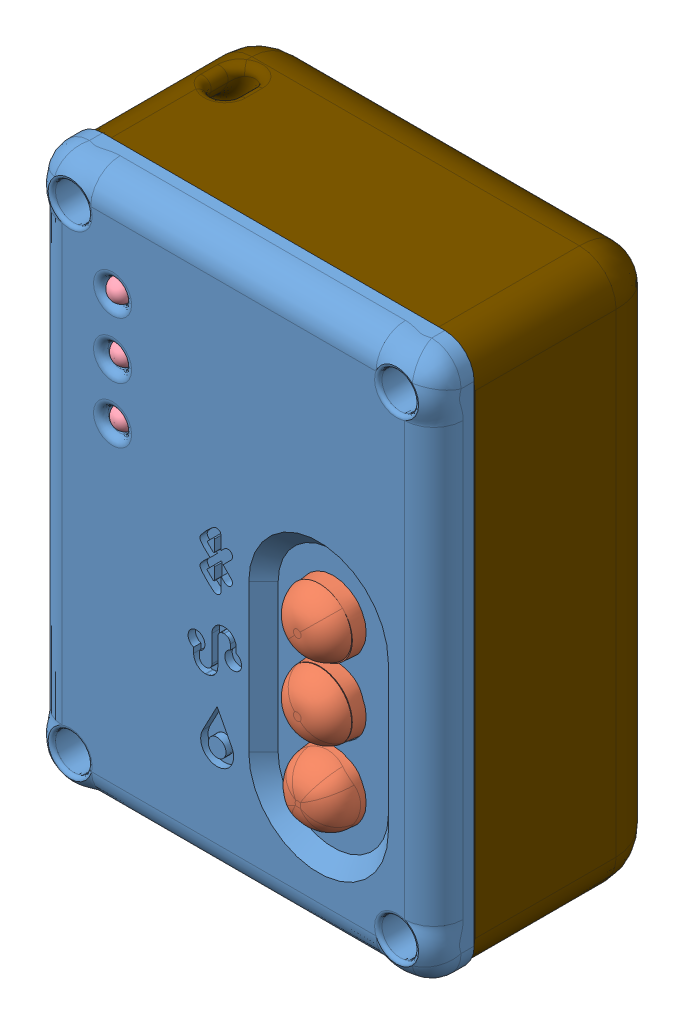
SolidWorks assembly tracker, configuration По умолчанию. Lengths in mm.
Overall size (452.18 452.18 291.35).
146 component instances, 27 part files, 100 mates.
Components (placement in the parent):
- YAAJ_BluePill.step-1: YAAJ_BluePill.step [По умолчанию] at origin size (22.6 53 12.5)
- Stiftleiste, RM 2,54 mm - 6-3 mm, gerade - 1 x 20 - schwarz.stp-3: Stiftleiste, RM 2,54 mm - 6-3 mm, gerade - 1 x 20 - schwarz.stp [По умолчанию] at (13.97 1.27 1.6) x (0 -1 0) z (0 0 1) size (50.8 2.54 11.57)
  - Stiftleiste, RM 2,54 mm - Tr_ger - 1 x 20 - schwarz.stp-1: Stiftleiste, RM 2,54 mm - Tr_ger - 1 x 20 - schwarz.stp [По умолчанию] at origin size (50.8 2.54 2.54)
  - Stiftleiste, RM 2,54 mm - Stift -  6-3 mm, gerade.stp-1: Stiftleiste, RM 2,54 mm - Stift -  6-3 mm, gerade.stp [По умолчанию] at (1.27 1.27 -3) size (1.03 1.03 11.57)
  - Stiftleiste, RM 2,54 mm - Stift -  6-3 mm, gerade.stp-2: Stiftleiste, RM 2,54 mm - Stift -  6-3 mm, gerade.stp [По умолчанию] at (46.99 1.27 -3) size (1.03 1.03 11.57)
  - Stiftleiste, RM 2,54 mm - Stift -  6-3 mm, gerade.stp-3: Stiftleiste, RM 2,54 mm - Stift -  6-3 mm, gerade.stp [По умолчанию] at (44.45 1.27 -3) size (1.03 1.03 11.57)
  - Stiftleiste, RM 2,54 mm - Stift -  6-3 mm, gerade.stp-4: Stiftleiste, RM 2,54 mm - Stift -  6-3 mm, gerade.stp [По умолчанию] at (41.91 1.27 -3) size (1.03 1.03 11.57)
  - Stiftleiste, RM 2,54 mm - Stift -  6-3 mm, gerade.stp-5: Stiftleiste, RM 2,54 mm - Stift -  6-3 mm, gerade.stp [По умолчанию] at (39.37 1.27 -3) size (1.03 1.03 11.57)
  - Stiftleiste, RM 2,54 mm - Stift -  6-3 mm, gerade.stp-6: Stiftleiste, RM 2,54 mm - Stift -  6-3 mm, gerade.stp [По умолчанию] at (36.83 1.27 -3) size (1.03 1.03 11.57)
  - Stiftleiste, RM 2,54 mm - Stift -  6-3 mm, gerade.stp-7: Stiftleiste, RM 2,54 mm - Stift -  6-3 mm, gerade.stp [По умолчанию] at (34.29 1.27 -3) size (1.03 1.03 11.57)
  - Stiftleiste, RM 2,54 mm - Stift -  6-3 mm, gerade.stp-8: Stiftleiste, RM 2,54 mm - Stift -  6-3 mm, gerade.stp [По умолчанию] at (31.75 1.27 -3) size (1.03 1.03 11.57)
  - Stiftleiste, RM 2,54 mm - Stift -  6-3 mm, gerade.stp-9: Stiftleiste, RM 2,54 mm - Stift -  6-3 mm, gerade.stp [По умолчанию] at (29.21 1.27 -3) size (1.03 1.03 11.57)
  - Stiftleiste, RM 2,54 mm - Stift -  6-3 mm, gerade.stp-10: Stiftleiste, RM 2,54 mm - Stift -  6-3 mm, gerade.stp [По умолчанию] at (49.53 1.27 -3) size (1.03 1.03 11.57)
  - Stiftleiste, RM 2,54 mm - Stift -  6-3 mm, gerade.stp-11: Stiftleiste, RM 2,54 mm - Stift -  6-3 mm, gerade.stp [По умолчанию] at (21.59 1.27 -3) size (1.03 1.03 11.57)
  - Stiftleiste, RM 2,54 mm - Stift -  6-3 mm, gerade.stp-12: Stiftleiste, RM 2,54 mm - Stift -  6-3 mm, gerade.stp [По умолчанию] at (19.05 1.27 -3) size (1.03 1.03 11.57)
  - Stiftleiste, RM 2,54 mm - Stift -  6-3 mm, gerade.stp-13: Stiftleiste, RM 2,54 mm - Stift -  6-3 mm, gerade.stp [По умолчанию] at (16.51 1.27 -3) size (1.03 1.03 11.57)
  - Stiftleiste, RM 2,54 mm - Stift -  6-3 mm, gerade.stp-14: Stiftleiste, RM 2,54 mm - Stift -  6-3 mm, gerade.stp [По умолчанию] at (6.35 1.27 -3) size (1.03 1.03 11.57)
  - Stiftleiste, RM 2,54 mm - Stift -  6-3 mm, gerade.stp-15: Stiftleiste, RM 2,54 mm - Stift -  6-3 mm, gerade.stp [По умолчанию] at (13.97 1.27 -3) size (1.03 1.03 11.57)
  - Stiftleiste, RM 2,54 mm - Stift -  6-3 mm, gerade.stp-16: Stiftleiste, RM 2,54 mm - Stift -  6-3 mm, gerade.stp [По умолчанию] at (11.43 1.27 -3) size (1.03 1.03 11.57)
  - Stiftleiste, RM 2,54 mm - Stift -  6-3 mm, gerade.stp-17: Stiftleiste, RM 2,54 mm - Stift -  6-3 mm, gerade.stp [По умолчанию] at (8.89 1.27 -3) size (1.03 1.03 11.57)
  - Stiftleiste, RM 2,54 mm - Stift -  6-3 mm, gerade.stp-18: Stiftleiste, RM 2,54 mm - Stift -  6-3 mm, gerade.stp [По умолчанию] at (26.67 1.27 -3) size (1.03 1.03 11.57)
  - Stiftleiste, RM 2,54 mm - Stift -  6-3 mm, gerade.stp-19: Stiftleiste, RM 2,54 mm - Stift -  6-3 mm, gerade.stp [По умолчанию] at (24.13 1.27 -3) size (1.03 1.03 11.57)
  - Stiftleiste, RM 2,54 mm - Stift -  6-3 mm, gerade.stp-20: Stiftleiste, RM 2,54 mm - Stift -  6-3 mm, gerade.stp [По умолчанию] at (3.81 1.27 -3) size (1.03 1.03 11.57)
- Stiftleiste, RM 2,54 mm - 6-3 mm, gerade - 1 x 20 - schwarz.stp-4: Stiftleiste, RM 2,54 mm - 6-3 mm, gerade - 1 x 20 - schwarz.stp [По умолчанию] at (1.27 -49.53 1.6) x (0 1 0) z (0 0 1) size (50.8 2.54 11.57)
  - Stiftleiste, RM 2,54 mm - Tr_ger - 1 x 20 - schwarz.stp-1: Stiftleiste, RM 2,54 mm - Tr_ger - 1 x 20 - schwarz.stp [По умолчанию] at origin size (50.8 2.54 2.54)
  - Stiftleiste, RM 2,54 mm - Stift -  6-3 mm, gerade.stp-1: Stiftleiste, RM 2,54 mm - Stift -  6-3 mm, gerade.stp [По умолчанию] at (1.27 1.27 -3) size (1.03 1.03 11.57)
  - Stiftleiste, RM 2,54 mm - Stift -  6-3 mm, gerade.stp-2: Stiftleiste, RM 2,54 mm - Stift -  6-3 mm, gerade.stp [По умолчанию] at (46.99 1.27 -3) size (1.03 1.03 11.57)
  - Stiftleiste, RM 2,54 mm - Stift -  6-3 mm, gerade.stp-3: Stiftleiste, RM 2,54 mm - Stift -  6-3 mm, gerade.stp [По умолчанию] at (44.45 1.27 -3) size (1.03 1.03 11.57)
  - Stiftleiste, RM 2,54 mm - Stift -  6-3 mm, gerade.stp-4: Stiftleiste, RM 2,54 mm - Stift -  6-3 mm, gerade.stp [По умолчанию] at (41.91 1.27 -3) size (1.03 1.03 11.57)
  - Stiftleiste, RM 2,54 mm - Stift -  6-3 mm, gerade.stp-5: Stiftleiste, RM 2,54 mm - Stift -  6-3 mm, gerade.stp [По умолчанию] at (39.37 1.27 -3) size (1.03 1.03 11.57)
  - Stiftleiste, RM 2,54 mm - Stift -  6-3 mm, gerade.stp-6: Stiftleiste, RM 2,54 mm - Stift -  6-3 mm, gerade.stp [По умолчанию] at (36.83 1.27 -3) size (1.03 1.03 11.57)
  - Stiftleiste, RM 2,54 mm - Stift -  6-3 mm, gerade.stp-7: Stiftleiste, RM 2,54 mm - Stift -  6-3 mm, gerade.stp [По умолчанию] at (34.29 1.27 -3) size (1.03 1.03 11.57)
  - Stiftleiste, RM 2,54 mm - Stift -  6-3 mm, gerade.stp-8: Stiftleiste, RM 2,54 mm - Stift -  6-3 mm, gerade.stp [По умолчанию] at (31.75 1.27 -3) size (1.03 1.03 11.57)
  - Stiftleiste, RM 2,54 mm - Stift -  6-3 mm, gerade.stp-9: Stiftleiste, RM 2,54 mm - Stift -  6-3 mm, gerade.stp [По умолчанию] at (29.21 1.27 -3) size (1.03 1.03 11.57)
  - Stiftleiste, RM 2,54 mm - Stift -  6-3 mm, gerade.stp-10: Stiftleiste, RM 2,54 mm - Stift -  6-3 mm, gerade.stp [По умолчанию] at (49.53 1.27 -3) size (1.03 1.03 11.57)
  - Stiftleiste, RM 2,54 mm - Stift -  6-3 mm, gerade.stp-11: Stiftleiste, RM 2,54 mm - Stift -  6-3 mm, gerade.stp [По умолчанию] at (21.59 1.27 -3) size (1.03 1.03 11.57)
  - Stiftleiste, RM 2,54 mm - Stift -  6-3 mm, gerade.stp-12: Stiftleiste, RM 2,54 mm - Stift -  6-3 mm, gerade.stp [По умолчанию] at (19.05 1.27 -3) size (1.03 1.03 11.57)
  - Stiftleiste, RM 2,54 mm - Stift -  6-3 mm, gerade.stp-13: Stiftleiste, RM 2,54 mm - Stift -  6-3 mm, gerade.stp [По умолчанию] at (16.51 1.27 -3) size (1.03 1.03 11.57)
  - Stiftleiste, RM 2,54 mm - Stift -  6-3 mm, gerade.stp-14: Stiftleiste, RM 2,54 mm - Stift -  6-3 mm, gerade.stp [По умолчанию] at (6.35 1.27 -3) size (1.03 1.03 11.57)
  - Stiftleiste, RM 2,54 mm - Stift -  6-3 mm, gerade.stp-15: Stiftleiste, RM 2,54 mm - Stift -  6-3 mm, gerade.stp [По умолчанию] at (13.97 1.27 -3) size (1.03 1.03 11.57)
  - Stiftleiste, RM 2,54 mm - Stift -  6-3 mm, gerade.stp-16: Stiftleiste, RM 2,54 mm - Stift -  6-3 mm, gerade.stp [По умолчанию] at (11.43 1.27 -3) size (1.03 1.03 11.57)
  - Stiftleiste, RM 2,54 mm - Stift -  6-3 mm, gerade.stp-17: Stiftleiste, RM 2,54 mm - Stift -  6-3 mm, gerade.stp [По умолчанию] at (8.89 1.27 -3) size (1.03 1.03 11.57)
  - Stiftleiste, RM 2,54 mm - Stift -  6-3 mm, gerade.stp-18: Stiftleiste, RM 2,54 mm - Stift -  6-3 mm, gerade.stp [По умолчанию] at (26.67 1.27 -3) size (1.03 1.03 11.57)
  - Stiftleiste, RM 2,54 mm - Stift -  6-3 mm, gerade.stp-19: Stiftleiste, RM 2,54 mm - Stift -  6-3 mm, gerade.stp [По умолчанию] at (24.13 1.27 -3) size (1.03 1.03 11.57)
  - Stiftleiste, RM 2,54 mm - Stift -  6-3 mm, gerade.stp-20: Stiftleiste, RM 2,54 mm - Stift -  6-3 mm, gerade.stp [По умолчанию] at (3.81 1.27 -3) size (1.03 1.03 11.57)
- pcb_proto_board(40x60) .step-1: pcb_proto_board(40x60) .step [По умолчанию] at (-10.994 5.734 9.14) x (0 -1 0) z (0 0 1) size (60 40 2.1)
- HC-05-1: HC-05 [Default] at (1.6677 -8.4393 11.13) x (0 -1 0) z (-1 0 0) size (42.58 5.8 16)
- Troyka SD card.stp-1: Troyka SD card.stp [По умолчанию] at (-11.7222 -53.8342 13.43) size (26.65 26.3 12.48)
  - SOT23-5.stp-1: SOT23-5.stp [По умолчанию] at (18.8632 22.6732 0.75) x (-1 0 0) z (0 0 1) size (3.1 3.38 1.3)
    - SOT23-5 Geometry.stp-1: SOT23-5 Geometry.stp [По умолчанию] at origin size (3.1 1.8 1.3)
    - leg.stp-1: leg.stp [По умолчанию] at origin size (0.5 0.79 1)
    - leg.stp-2: leg.stp [По умолчанию] at (-0.95 0 0) size (0.5 0.79 1)
    - leg.stp-3: leg.stp [По умолчанию] at (-1.9 0 0) size (0.5 0.79 1)
    - leg.stp-4: leg.stp [По умолчанию] at (0 0.01 0) x (-1 0 0) z (0 0 1) size (0.5 0.79 1)
    - leg.stp-5: leg.stp [По умолчанию] at (1.9 0.01 0) x (-1 0 0) z (0 0 1) size (0.5 0.79 1)
  - SOT23-5-1.stp-1: SOT23-5-1.stp [По умолчанию] at (11.4972 22.8002 0.75) x (-1 0 0) z (0 0 1) size (3.1 3.38 1.3)
    - SOT23-5 Geometry.stp-1: SOT23-5 Geometry.stp [По умолчанию] at origin size (3.1 1.8 1.3)
    - leg.stp-1: leg.stp [По умолчанию] at origin size (0.5 0.79 1)
    - leg.stp-2: leg.stp [По умолчанию] at (-0.95 0 0) size (0.5 0.79 1)
    - leg.stp-3: leg.stp [По умолчанию] at (-1.9 0 0) size (0.5 0.79 1)
    - leg.stp-4: leg.stp [По умолчанию] at (0 0.01 0) x (-1 0 0) z (0 0 1) size (0.5 0.79 1)
    - leg.stp-5: leg.stp [По умолчанию] at (1.9 0.01 0) x (-1 0 0) z (0 0 1) size (0.5 0.79 1)
  - SOT23-5-2.stp-1: SOT23-5-2.stp [По умолчанию] at (15.1802 22.4192 0.75) x (-1 0 0) z (0 0 1) size (3.1 3.38 1.3)
    - SOT23-5 Geometry.stp-1: SOT23-5 Geometry.stp [По умолчанию] at origin size (3.1 1.8 1.3)
    - leg.stp-1: leg.stp [По умолчанию] at origin size (0.5 0.79 1)
    - leg.stp-2: leg.stp [По умолчанию] at (-0.95 0 0) size (0.5 0.79 1)
    - leg.stp-3: leg.stp [По умолчанию] at (-1.9 0 0) size (0.5 0.79 1)
    - leg.stp-4: leg.stp [По умолчанию] at (0 0.01 0) x (-1 0 0) z (0 0 1) size (0.5 0.79 1)
    - leg.stp-5: leg.stp [По умолчанию] at (1.9 0.01 0) x (-1 0 0) z (0 0 1) size (0.5 0.79 1)
  - SOT23-5-3.stp-1: SOT23-5-3.stp [По умолчанию] at (22.6732 7.4332 0.75) x (0 -1 0) z (0 0 1) size (3.1 3.38 1.3)
    - SOT23-5 Geometry.stp-1: SOT23-5 Geometry.stp [По умолчанию] at origin size (3.1 1.8 1.3)
    - leg.stp-1: leg.stp [По умолчанию] at origin size (0.5 0.79 1)
    - leg.stp-2: leg.stp [По умолчанию] at (-0.95 0 0) size (0.5 0.79 1)
    - leg.stp-3: leg.stp [По умолчанию] at (-1.9 0 0) size (0.5 0.79 1)
    - leg.stp-4: leg.stp [По умолчанию] at (0 0.01 0) x (-1 0 0) z (0 0 1) size (0.5 0.79 1)
    - leg.stp-5: leg.stp [По умолчанию] at (1.9 0.01 0) x (-1 0 0) z (0 0 1) size (0.5 0.79 1)
  - SOT23-5-4.stp-1: SOT23-5-4.stp [По умолчанию] at (2.9882 19.4982 0.75) size (3.1 3.38 1.3)
    - SOT23-5 Geometry.stp-1: SOT23-5 Geometry.stp [По умолчанию] at origin size (3.1 1.8 1.3)
    - leg.stp-1: leg.stp [По умолчанию] at origin size (0.5 0.79 1)
    - leg.stp-2: leg.stp [По умолчанию] at (-0.95 0 0) size (0.5 0.79 1)
    - leg.stp-3: leg.stp [По умолчанию] at (-1.9 0 0) size (0.5 0.79 1)
    - leg.stp-4: leg.stp [По умолчанию] at (0 0.01 0) x (-1 0 0) z (0 0 1) size (0.5 0.79 1)
    - leg.stp-5: leg.stp [По умолчанию] at (1.9 0.01 0) x (-1 0 0) z (0 0 1) size (0.5 0.79 1)
  - 1X03_soldered.stp-1: 1X03_soldered.stp [По умолчанию] at (4.2582 13.1482 -0.75) x (0 -1 0) z (0 0 -1) size (7.62 2.54 10.16)
    - PLS 1x1_soldered.stp-1: PLS 1x1_soldered.stp [По умолчанию] at (2.54 -6.35 0) x (0 1 0) z (0 0 1) size (2.54 2.54 10.16)
      - PLS 1x1_soldered Geometry.stp-1: PLS 1x1_soldered Geometry.stp [По умолчанию] at origin size (2.54 2.54 10.16)
      - Component29.stp-1: Component29.stp [По умолчанию] at (6.35 0 0) size (2.11 2.11 0.87)
    - PLS 1x1_soldered-1.stp-1: PLS 1x1_soldered-1.stp [По умолчанию] at (0 -6.35 0) x (0 1 0) z (0 0 1) size (2.54 2.54 10.16)
      - PLS 1x1_soldered Geometry.stp-1: PLS 1x1_soldered Geometry.stp [По умолчанию] at origin size (2.54 2.54 10.16)
      - Component29.stp-1: Component29.stp [По умолчанию] at (6.35 0 0) size (2.11 2.11 0.87)
    - PLS 1x1_soldered-2.stp-1: PLS 1x1_soldered-2.stp [По умолчанию] at (-2.54 -6.35 0) x (0 1 0) z (0 0 1) size (2.54 2.54 10.16)
      - PLS 1x1_soldered Geometry.stp-1: PLS 1x1_soldered Geometry.stp [По умолчанию] at origin size (2.54 2.54 10.16)
      - Component29.stp-1: Component29.stp [По умолчанию] at (6.35 0 0) size (2.11 2.11 0.87)
  - 1X03_soldered-1.stp-1: 1X03_soldered-1.stp [По умолчанию] at (22.0382 13.1482 -0.75) x (0 -1 0) z (0 0 -1) size (7.62 2.54 10.16)
    - PLS 1x1_soldered-3.stp-1: PLS 1x1_soldered-3.stp [По умолчанию] at (2.54 -6.35 0) x (0 1 0) z (0 0 1) size (2.54 2.54 10.16)
      - PLS 1x1_soldered Geometry.stp-1: PLS 1x1_soldered Geometry.stp [По умолчанию] at origin size (2.54 2.54 10.16)
      - Component29.stp-1: Component29.stp [По умолчанию] at (6.35 0 0) size (2.11 2.11 0.87)
    - PLS 1x1_soldered-4.stp-1: PLS 1x1_soldered-4.stp [По умолчанию] at (0 -6.35 0) x (0 1 0) z (0 0 1) size (2.54 2.54 10.16)
      - PLS 1x1_soldered Geometry.stp-1: PLS 1x1_soldered Geometry.stp [По умолчанию] at origin size (2.54 2.54 10.16)
      - Component29.stp-1: Component29.stp [По умолчанию] at (6.35 0 0) size (2.11 2.11 0.87)
    - PLS 1x1_soldered-5.stp-1: PLS 1x1_soldered-5.stp [По умолчанию] at (-2.54 -6.35 0) x (0 1 0) z (0 0 1) size (2.54 2.54 10.16)
      - PLS 1x1_soldered Geometry.stp-1: PLS 1x1_soldered Geometry.stp [По умолчанию] at origin size (2.54 2.54 10.16)
      - Component29.stp-1: Component29.stp [По умолчанию] at (6.35 0 0) size (2.11 2.11 0.87)
  - Micro SD cardreader with SD.stp-1: Micro SD cardreader with SD.stp [По умолчанию] at (-184.7507 56.4832 123.6639) x (0 0 1) z (1 0 0) size (1.85 17.9 14.8)
    - Micro SD.stp-1: Micro SD.stp [По умолчанию] at (-120.5536 45.5089 151.9853) x (0 0 1) z (1 0 0) size (11 15 1.1)
    - slot.stp-1: slot.stp [По умолчанию] at (-120.5536 47.0914 197.6703) x (0 0 1) z (1 0 0) size (14.8 15 1.85)
  - C0603.stp-1: C0603.stp [По умолчанию] at (5.7822 20.0062 0.75) x (0 1 0) z (0 0 1) size (1.61 0.81 0.46)
  - C0603.stp-2: C0603.stp [По умолчанию] at (5.7822 23.3082 0.75) x (0 1 0) z (0 0 1) size (1.61 0.81 0.46)
  - C0603.stp-3: C0603.stp [По умолчанию] at (22.6732 4.6392 0.75) x (-1 0 0) z (0 0 1) size (1.61 0.81 0.46)
  - C0603.stp-4: C0603.stp [По умолчанию] at (7.8142 20.0062 0.75) x (0 -1 0) z (0 0 1) size (1.61 0.81 0.46)
  - C0603.stp-5: C0603.stp [По умолчанию] at (15.3072 19.2442 0.75) x (-1 0 0) z (0 0 1) size (1.61 0.81 0.46)
  - C0603.stp-6: C0603.stp [По умолчанию] at (18.7362 19.3712 0.75) x (-1 0 0) z (0 0 1) size (1.61 0.81 0.46)
  - R0603.stp-1: R0603.stp [По умолчанию] at (2.9882 6.1632 0.75) size (1.61 0.81 0.46)
  - R0603.stp-2: R0603.stp [По умолчанию] at (2.9882 8.0682 0.75) size (1.61 0.81 0.46)
  - R0603.stp-3: R0603.stp [По умолчанию] at (7.8142 23.3082 0.75) x (0 1 0) z (0 0 1) size (1.61 0.81 0.46)
  - R0603.stp-4: R0603.stp [По умолчанию] at (22.6732 20.7682 0.75) size (1.61 0.81 0.46)
  - R0603.stp-5: R0603.stp [По умолчанию] at (22.6732 18.7362 0.75) x (-1 0 0) z (0 0 1) size (1.61 0.81 0.46)
  - R0603.stp-6: R0603.stp [По умолчанию] at (11.4972 19.4982 0.75) size (1.61 0.81 0.46)
  - pcbgroup.stp-1: pcbgroup.stp [По умолчанию] at (0.4482 25.8482 -0.75) x (0 -1 0) z (0 0 1) size (25.4 25.4 1.5)
- tp4056 micro usb 18650 charger-1: tp4056 micro usb 18650 charger [Výchozí] at (-2.344 -40.316 4.64) x (-1 0 0) z (0 0 -1) size (17.3 29.2 4)
- ADTS648SV.step-1: ADTS648SV.step [По умолчанию] at (20.516 -44.466 11.14) x (0 -1 0) z (0 0 1) size (8.12 6.2 10.85)
- ADTS648SV.step-2: ADTS648SV.step [По умолчанию] at (20.516 -34.366 11.14) x (0 1 0) z (0 0 1) size (8.12 6.2 10.85)
- ADTS648SV.step-3: ADTS648SV.step [По умолчанию] at (20.516 -24.366 11.14) x (0 1 0) z (0 0 1) size (8.12 6.2 10.85)
- аккумулятор-1: аккумулятор [По умолчанию] at (26.006 -49.266 -2) x (0 1 0) z (0 0 -1) size (50 34 3.8)
- Деталь1^tracker-1: Деталь1^tracker [По умолчанию] at (26.006 -49.266 -5.8) x (0 1 0) z (0 0 -1) size (74.6 74.6 46.24) (virtual)
- Деталь2^tracker-1: Деталь2^tracker [По умолчанию] at (40.1615 -43.814 18.24) x (0 -1 0) z (0 0 1) size (94.6 74.6 8.6) (virtual)
- Деталь4^tracker-1: Деталь4^tracker [По умолчанию] at (40.1615 -43.814 19.74) x (0 -1 0) z (0 0 1) size (30 10 12.41) (virtual)
- кнопка включения-1: кнопка включения [По умолчанию] at (-12.294 -42.566 -4) x (0 1 0) z (-1 0 0) size (36 8 7.5)
- LED 3mm Red 3mm Leads.step-1: LED 3mm Red 3mm Leads.step [По умолчанию] at (-7.5324 0.3024 16.63) size (3.45 3.85 8.38)
  - LEDBody.step-1: LEDBody.step [По умолчанию] at (0 0 0.01) size (3.45 3.85 5.38)
  - Lead1Body.step-1: Lead1Body.step [По умолчанию] at (0 0 0.01) size (0.5 0.5 3)
  - Lead2Body.step-1: Lead2Body.step [По умолчанию] at (0 0 0.01) size (0.5 0.5 3)
- LED 3mm Red 3mm Leads.step-2: LED 3mm Red 3mm Leads.step [По умолчанию] at (-7.5324 -14.9883 16.13) size (3.45 3.85 8.38)
  - LEDBody.step-1: LEDBody.step [По умолчанию] at (0 0 0.01) size (3.45 3.85 5.38)
  - Lead1Body.step-1: Lead1Body.step [По умолчанию] at (0 0 0.01) size (0.5 0.5 3)
  - Lead2Body.step-1: Lead2Body.step [По умолчанию] at (0 0 0.01) size (0.5 0.5 3)
- LED 3mm Red 3mm Leads.step-3: LED 3mm Red 3mm Leads.step [По умолчанию] at (-7.5324 -7.3883 16.13) size (3.45 3.85 8.38)
  - LEDBody.step-1: LEDBody.step [По умолчанию] at (0 0 0.01) size (3.45 3.85 5.38)
  - Lead1Body.step-1: Lead1Body.step [По умолчанию] at (0 0 0.01) size (0.5 0.5 3)
  - Lead2Body.step-1: Lead2Body.step [По умолчанию] at (0 0 0.01) size (0.5 0.5 3)
- прокладка-1: прокладка [По умолчанию] at (9.006 -24.266 16.24) x (0 -1 0) z (0 0 1) size (72.4 52.4 1.8)
- Деталь3^tracker-1: Деталь3^tracker [По умолчанию] at (26.006 -61.566 -5.8) x (0 0 -1) z (0 -1 0) size (9.6 14.6 9) (virtual)
- M2 x 5 Screw head.step-1: M2 x 5 Screw head.step [По умолчанию] at (31.1444 -56.4044 18.84) x (0 0 -1) z (1 0 0) size (6.58 4 4)
- M2 x 5 Screw head.step-2: M2 x 5 Screw head.step [По умолчанию] at (-13.3092 -56.7812 18.84) x (0 0 -1) z (0 -1 0) size (6.58 4 4)
- M2 x 5 Screw head.step-3: M2 x 5 Screw head.step [По умолчанию] at (-13.3092 8.0492 18.84) x (0 0 -1) z (1 0 0) size (6.58 4 4)
- M2 x 5 Screw head.step-4: M2 x 5 Screw head.step [По умолчанию] at (31.1444 8.0492 18.84) x (0 0 -1) z (0 1 0) size (6.58 4 4)
Mates (geometry in assembly coordinates):
- Совпадение1: coincident anti-aligned: plane of YAAJ_BluePill.step-1 through (7.62 -24.13 1.6) normal (0 0 1); plane of Stiftleiste, RM 2,54 mm - 6-3 mm, gerade - 1 x 20 - schwarz.stp-3/Stiftleiste, RM 2,54 mm - Tr_ger - 1 x 20 - schwarz.stp-1 through (13.97 1.27 1.6) normal (0 0 -1)
- Параллельность8: parallel anti-aligned: plane of YAAJ_BluePill.step-1 through (18.92 -50.63 1.6) normal (1 0 0); plane of Stiftleiste, RM 2,54 mm - 6-3 mm, gerade - 1 x 20 - schwarz.stp-3/Stiftleiste, RM 2,54 mm - Tr_ger - 1 x 20 - schwarz.stp-1 through (13.97 1.27 4.14) normal (-1 0 0)
- Концентричный1: concentric aligned: cylinder of YAAJ_BluePill.step-1 through (15.24 -48.26 -0.001) axis (0 0 1) radius 0.4995; cylinder of Stiftleiste, RM 2,54 mm - 6-3 mm, gerade - 1 x 20 - schwarz.stp-3/Stiftleiste, RM 2,54 mm - Stift -  6-3 mm, gerade.stp-10 through (15.24 -48.26 -1.4) axis (0 0 1) radius 0.5
- Совпадение3: coincident anti-aligned: plane of YAAJ_BluePill.step-1 through (7.62 -24.13 1.6) normal (0 0 1); plane of Stiftleiste, RM 2,54 mm - 6-3 mm, gerade - 1 x 20 - schwarz.stp-4/Stiftleiste, RM 2,54 mm - Tr_ger - 1 x 20 - schwarz.stp-1 through (1.27 -49.53 1.6) normal (0 0 -1)
- Параллельность9: parallel anti-aligned: plane of YAAJ_BluePill.step-1 through (-3.68 2.37 1.6) normal (-1 0 0); plane of Stiftleiste, RM 2,54 mm - 6-3 mm, gerade - 1 x 20 - schwarz.stp-4/Stiftleiste, RM 2,54 mm - Tr_ger - 1 x 20 - schwarz.stp-1 through (1.27 -49.53 4.14) normal (1 0 0)
- Концентричный2: concentric aligned: cylinder of YAAJ_BluePill.step-1 through (0 -48.26 -0.001) axis (0 0 1) radius 0.4995; cylinder of Stiftleiste, RM 2,54 mm - 6-3 mm, gerade - 1 x 20 - schwarz.stp-4/Stiftleiste, RM 2,54 mm - Stift -  6-3 mm, gerade.stp-1 through (0 -48.26 -1.4) axis (0 0 1) radius 0.5
- Параллельность10: parallel anti-aligned: plane of YAAJ_BluePill.step-1 through (-3.68 2.37 1.6) normal (-1 0 0); plane of pcb_proto_board(40x60) .step-1 through (29.006 -54.266 9.14) normal (1 0 0)
- Расстояние2: distance = 4 mm anti-aligned: plane of pcb_proto_board(40x60) .step-1 through (9.006 -24.266 8.14) normal (0 0 -1); plane of Stiftleiste, RM 2,54 mm - 6-3 mm, gerade - 1 x 20 - schwarz.stp-4/Stiftleiste, RM 2,54 mm - Tr_ger - 1 x 20 - schwarz.stp-1 through (1.27 -49.53 4.14) normal (0 0 1)
- Концентричный3: concentric anti-aligned: cylinder of Stiftleiste, RM 2,54 mm - 6-3 mm, gerade - 1 x 20 - schwarz.stp-3/Stiftleiste, RM 2,54 mm - Stift -  6-3 mm, gerade.stp-10 through (15.24 -48.26 -1.4) axis (0 0 1) radius 0.5; circle of pcb_proto_board(40x60) .step-1
- Параллельность11: parallel aligned: plane of pcb_proto_board(40x60) .step-1 through (-10.994 5.734 9.14) normal (-1 0 0); plane of HC-05-1 through (-6.3323 -26.9393 12.43) normal (-1 0 0)
- Параллельность12: parallel anti-aligned: plane of pcb_proto_board(40x60) .step-1 through (9.006 -24.266 10.14) normal (0 0 1); plane of HC-05-1 through (1.6677 -8.4393 11.13) normal (0 0 -1)
- Расстояние3: distance = 1 mm anti-aligned: plane of HC-05-1 through (1.6677 -8.4393 11.14) normal (0 0 -1); plane of pcb_proto_board(40x60) .step-1 through (9.006 -24.266 10.14) normal (0 0 1)
- Параллельность13: parallel aligned: plane of pcb_proto_board(40x60) .step-1 through (-10.994 5.734 9.14) normal (-1 0 0); plane of Troyka SD card.stp-1/pcbgroup.stp-1 through (-11.274 -40.686 14.18) normal (-1 0 0)
- Концентричный7: concentric anti-aligned: cylinder of pcb_proto_board(40x60) .step-1 through (-4.968 -25.526 10.14) axis (0 0 -1) radius 0.5; cylinder of HC-05-1 through (-4.968 -25.526 10.63) axis (0 0 1) radius 0.4016
- Расстояние4: distance = 3.23 mm aligned: plane of Troyka SD card.stp-1/1X03_soldered.stp-1/PLS 1x1_soldered.stp-1/PLS 1x1_soldered Geometry.stp-1 through (-7.764 -43.526 7.847) normal (-1 0 0); plane of pcb_proto_board(40x60) .step-1 through (-10.994 5.734 9.14) normal (-1 0 0)
- Расстояние5: distance = 10.74 mm aligned: plane of Troyka SD card.stp-1/1X03_soldered.stp-1/PLS 1x1_soldered.stp-1/PLS 1x1_soldered Geometry.stp-1 through (-6.194 -43.526 12.68) normal (0 -1 0); plane of pcb_proto_board(40x60) .step-1 through (-10.994 -54.266 9.14) normal (0 -1 0)
- Совпадение11: coincident anti-aligned: plane of pcb_proto_board(40x60) .step-1 through (9.006 -24.266 10.14) normal (0 0 1); plane of Troyka SD card.stp-1/1X03_soldered.stp-1/PLS 1x1_soldered-2.stp-1/PLS 1x1_soldered Geometry.stp-1 through (-6.194 -39.416 10.14) normal (0 0 -1)
- Параллельность14: parallel anti-aligned: plane of pcb_proto_board(40x60) .step-1 through (29.006 -54.266 9.14) normal (1 0 0); plane of tp4056 micro usb 18650 charger-1 through (-10.994 -40.316 5.74) normal (-1 0 0)
- Параллельность15: parallel aligned: plane of pcb_proto_board(40x60) .step-1 through (9.006 -24.266 10.14) normal (0 0 1); plane of tp4056 micro usb 18650 charger-1 through (-2.344 -40.316 5.74) normal (0 0 1)
- Расстояние7: distance = 1 mm anti-aligned: plane of ADTS648SV.step-1 through (20.516 -44.466 11.14) normal (0 0 -1); plane of pcb_proto_board(40x60) .step-1 through (9.006 -24.266 10.14) normal (0 0 1)
- Параллельность17: parallel anti-aligned: plane of pcb_proto_board(40x60) .step-1 through (29.006 -54.266 9.14) normal (1 0 0); plane of ADTS648SV.step-1 through (17.416 -41.366 11.14) normal (-1 0 0)
- Расстояние11: distance = 5.39 mm aligned: plane of ADTS648SV.step-1 through (23.616 -47.566 11.14) normal (1 0 0); plane of pcb_proto_board(40x60) .step-1 through (29.006 -54.266 9.14) normal (1 0 0)
- Расстояние12: distance = 6.7 mm aligned: plane of ADTS648SV.step-1 through (17.416 -47.566 11.14) normal (0 -1 0); plane of pcb_proto_board(40x60) .step-1 through (-10.994 -54.266 9.14) normal (0 -1 0)
- Параллельность18: parallel anti-aligned: plane of pcb_proto_board(40x60) .step-1 through (9.006 -24.266 10.14) normal (0 0 1); plane of ADTS648SV.step-2 through (20.516 -34.366 11.14) normal (0 0 -1)
- Расстояние13: distance = 1 mm anti-aligned: plane of ADTS648SV.step-2 through (20.516 -34.366 11.14) normal (0 0 -1); plane of pcb_proto_board(40x60) .step-1 through (9.006 -24.266 10.14) normal (0 0 1)
- Расстояние15: distance = 5.39 mm aligned: plane of ADTS648SV.step-2 through (23.616 -37.466 11.14) normal (1 0 0); plane of pcb_proto_board(40x60) .step-1 through (29.006 -54.266 9.14) normal (1 0 0)
- Расстояние17: distance = 16.8 mm aligned: plane of ADTS648SV.step-2 through (17.416 -37.466 11.14) normal (0 -1 0); plane of pcb_proto_board(40x60) .step-1 through (-10.994 -54.266 9.14) normal (0 -1 0)
- Параллельность19: parallel anti-aligned: plane of pcb_proto_board(40x60) .step-1 through (9.006 -24.266 10.14) normal (0 0 1); plane of ADTS648SV.step-3 through (20.516 -24.366 11.14) normal (0 0 -1)
- Расстояние18: distance = 1 mm anti-aligned: plane of ADTS648SV.step-3 through (20.516 -24.366 11.14) normal (0 0 -1); plane of pcb_proto_board(40x60) .step-1 through (9.006 -24.266 10.14) normal (0 0 1)
- Расстояние22: distance = 33 mm anti-aligned: plane of ADTS648SV.step-3 through (23.616 -21.266 11.14) normal (0 1 0); plane of pcb_proto_board(40x60) .step-1 through (-10.994 -54.266 9.14) normal (0 -1 0)
- Параллельность20: parallel anti-aligned: plane of pcb_proto_board(40x60) .step-1 through (9.006 -24.266 8.14) normal (0 0 -1); plane of аккумулятор-1 through (26.006 -49.266 -2) normal (0 0 1)
- Расстояние24: distance = 3 mm aligned: plane of аккумулятор-1 through (-7.994 -49.266 -5.8) normal (-1 0 0); plane of pcb_proto_board(40x60) .step-1 through (-10.994 5.734 9.14) normal (-1 0 0)
- Расстояние25: distance = 2 mm anti-aligned: plane of аккумулятор-1 through (26.006 -49.266 -2) normal (0 0 1); plane of YAAJ_BluePill.step-1 through (7.62 -24.13 0) normal (0 0 -1)
- Расстояние26: distance = 5 mm aligned: plane of аккумулятор-1 through (26.006 -49.266 -5.8) normal (0 -1 0); plane of pcb_proto_board(40x60) .step-1 through (-10.994 -54.266 9.14) normal (0 -1 0)
- На месте1: in place: plane of аккумулятор-1 through (26.006 -49.266 -5.8) normal (0 0 -1); plane of ? through (0 0 -5.8) normal (0 0 -1); moOrthogonalPlaneRef_w of аккумулятор-1 through (26.006 -49.266 -5.8) normal (0 0 -1); plane of ? through (0 0 -5.8) normal (0 1 0); plane of аккумулятор-1 through (26.006 -49.266 -5.8) normal (0 0 -1); plane of ? through (0 0 -5.8) normal (-1 0 0); plane of аккумулятор-1 through (26.006 -49.266 -5.8) normal (0 0 -1); unknown of Деталь1^tracker-1
- Совпадение40: coincident aligned: plane of аккумулятор-1; plane of Деталь1^tracker-1
- Совпадение41: coincident aligned: moOrthogonalPlaneRef_w of аккумулятор-1 through (26.006 -49.266 -5.8) normal (1 0 0); plane of Деталь1^tracker-1 through (26.006 -49.266 -5.8) normal (1 0 0)
- Совпадение42: coincident anti-aligned: moOrthogonalPlaneRef_w of аккумулятор-1 through (26.006 -49.266 -5.8) normal (0 -1 0); plane of Деталь1^tracker-1 through (26.006 -49.266 -5.8) normal (0 1 0)
- Совпадение15: coincident anti-aligned: plane of Деталь1^tracker-1 through (26.006 -49.266 16.24) normal (0 0 1); plane of Деталь2^tracker-1 through (40.1615 -43.814 16.24) normal (0 0 -1)
- Совпадение16: coincident aligned: plane of Деталь1^tracker-1 through (-16.294 -54.566 -6) normal (-1 0 0); plane of Деталь2^tracker-1 through (-16.294 11.034 18.74) normal (-1 0 0)
- Совпадение17: coincident aligned: plane of Деталь1^tracker-1 through (29.306 -59.566 -6) normal (0 -1 0); plane of Деталь2^tracker-1 through (-16.294 -59.566 18.74) normal (0 -1 0)
- Расстояние27: distance = 10.69 mm aligned: plane of Деталь1^tracker-1 through (34.306 6.034 -6) normal (1 0 0); plane of ADTS648SV.step-3 through (23.616 -27.466 11.14) normal (1 0 0)
- На месте3: in place: plane of ? through (40.2499 -43.9023 19.74) normal (0 0 1); plane of ? through (0 0 19.74) normal (0 0 1); plane of ? through (40.2499 -43.9023 19.74) normal (0 0 1); plane of ? through (0 0 19.74) normal (0 1 0); plane of ? through (40.2499 -43.9023 19.74) normal (0 0 1); plane of ? through (0 0 19.74) normal (1 0 0); plane of Деталь2^tracker-1 through (40.1615 -43.814 19.74) normal (0 0 1); unknown of Деталь4^tracker-1
- Совпадение19: coincident aligned: plane of Деталь2^tracker-1; plane of Деталь4^tracker-1
- Совпадение20: coincident aligned: moOrthogonalPlaneRef_w of Деталь2^tracker-1 through (40.1615 -43.814 19.74) normal (1 0 0); plane of Деталь4^tracker-1 through (40.1615 -43.814 19.74) normal (1 0 0)
- Совпадение21: coincident anti-aligned: moOrthogonalPlaneRef_w of Деталь2^tracker-1 through (40.1615 -43.814 19.74) normal (0 1 0); plane of Деталь4^tracker-1 through (40.1615 -43.814 19.74) normal (0 -1 0)
- Параллельность21: parallel anti-aligned: plane of pcb_proto_board(40x60) .step-1 through (9.006 -24.266 10.14) normal (0 0 1); plane of LED 5mm.step-1 through (-7.444 -1.486 13.24) normal (0 0 -1)
- Совпадение19: coincident anti-aligned: plane of Деталь2^tracker-1 through (40.1615 -43.814 21.74) normal (0 0 1); point of LED 5mm.step-1
- Параллельность22: parallel anti-aligned: plane of pcb_proto_board(40x60) .step-1 through (-10.994 5.734 9.14) normal (-1 0 0); plane of LED 5mm.step-1 through (-7.194 0.034 -14.76) normal (1 0 0)
- Расстояние28: distance = 3.3 mm aligned: plane of LED 5mm.step-1 through (-7.694 -2.506 -14.76) normal (-1 0 0); plane of pcb_proto_board(40x60) .step-1 through (-10.994 5.734 9.14) normal (-1 0 0)
- Расстояние29: distance = 5.7 mm aligned: plane of LED 5mm.step-1 through (-7.694 0.034 -14.76) normal (0 1 0); plane of pcb_proto_board(40x60) .step-1 through (29.006 5.734 9.14) normal (0 1 0)
- Параллельность23: parallel anti-aligned: plane of pcb_proto_board(40x60) .step-1 through (9.006 -24.266 10.14) normal (0 0 1); plane of LED 5mm.step-2 through (-7.444 -9.086 13.24) normal (0 0 -1)
- Параллельность24: parallel aligned: plane of pcb_proto_board(40x60) .step-1 through (-10.994 5.734 9.14) normal (-1 0 0); plane of LED 5mm.step-2 through (-7.694 -7.566 -14.76) normal (-1 0 0)
- Совпадение27: coincident: plane of Деталь2^tracker-1 through (40.1615 -43.814 21.74) normal (0 0 1); point of LED 5mm.step-2
- Расстояние30: distance = 0 mm aligned: plane of LED 5mm.step-2 through (-7.694 -7.566 -14.76) normal (-1 0 0); plane of LED 5mm.step-1 through (-7.694 -2.506 -14.76) normal (-1 0 0)
- Расстояние31: distance = 13.3 mm aligned: plane of LED 5mm.step-2 through (-7.694 -7.566 -14.76) normal (0 1 0); plane of pcb_proto_board(40x60) .step-1 through (29.006 5.734 9.14) normal (0 1 0)
- Параллельность25: parallel anti-aligned: plane of pcb_proto_board(40x60) .step-1 through (9.006 -24.266 10.14) normal (0 0 1); plane of LED 5mm.step-3 through (-7.444 -16.686 13.24) normal (0 0 -1)
- Параллельность26: parallel aligned: plane of pcb_proto_board(40x60) .step-1 through (-10.994 5.734 9.14) normal (-1 0 0); plane of LED 5mm.step-3 through (-7.694 -15.166 -14.76) normal (-1 0 0)
- Расстояние32: distance = 0 mm aligned: plane of LED 5mm.step-3 through (-7.694 -15.166 -14.76) normal (-1 0 0); plane of LED 5mm.step-2 through (-7.694 -10.106 -14.76) normal (-1 0 0)
- Совпадение33: coincident: plane of Деталь2^tracker-1 through (40.1615 -43.814 21.74) normal (0 0 1); point of LED 5mm.step-3
- Расстояние33: distance = 20.9 mm aligned: plane of LED 5mm.step-3 through (-7.694 -15.166 -14.76) normal (0 1 0); plane of pcb_proto_board(40x60) .step-1 through (29.006 5.734 9.14) normal (0 1 0)
- На месте4: in place: plane of Деталь1^tracker-1 through (-11.294 11.034 -6) normal (0 1 0); plane of ? through (0 11.034 0) normal (0 1 0); plane of Деталь1^tracker-1 through (-11.294 11.034 -6) normal (0 1 0); plane of ? through (0 11.034 0) normal (0 0 -1); plane of Деталь1^tracker-1 through (-11.294 11.034 -6) normal (0 1 0); plane of ? through (0 11.034 0) normal (1 0 0); plane of Деталь1^tracker-1 through (-11.294 11.034 -6) normal (0 1 0); unknown of ?
- Совпадение34: coincident aligned: plane of Деталь1^tracker-1; plane of Деталь3^tracker-1
- Совпадение35: coincident aligned: moOrthogonalPlaneRef_w of Деталь1^tracker-1 through (26.006 11.034 -5.8) normal (1 0 0); plane of Деталь3^tracker-1 through (26.006 11.034 -5.8) normal (1 0 0)
- Совпадение36: coincident anti-aligned: moOrthogonalPlaneRef_w of Деталь1^tracker-1 through (26.006 11.034 -5.8) normal (0 0 -1); plane of Деталь3^tracker-1
- Совпадение34: coincident anti-aligned: circle of Деталь1^tracker-1; plane of кнопка включения-1 through (-16.294 -42.566 -4) normal (-1 0 0)
- Параллельность27: parallel anti-aligned: plane of Деталь1^tracker-1 through (26.006 -49.266 16.24) normal (0 0 1); plane of кнопка включения-1 through (-16.294 -42.566 -4) normal (0 0 -1)
- Концентричный11: concentric aligned: cylinder of Деталь1^tracker-1 through (-18.294 -36.566 0) axis (1 0 0) radius 3.65; cylinder of кнопка включения-1 through (-18.294 -36.566 0) axis (1 0 0) radius 3.75
- Совпадение37: coincident aligned: plane of pcb_proto_board(40x60) .step-1 through (-10.994 -54.266 9.14) normal (0 -1 0); plane of tp4056 micro usb 18650 charger-1 through (-2.344 -54.266 5.74) normal (0 -1 0)
- Совпадение38: coincident aligned: plane of pcb_proto_board(40x60) .step-1 through (-10.994 5.734 9.14) normal (-1 0 0); plane of tp4056 micro usb 18650 charger-1 through (-10.994 -40.316 5.74) normal (-1 0 0)
- Расстояние34: distance = 3.5 mm aligned: plane of pcb_proto_board(40x60) .step-1 through (9.006 -24.266 8.14) normal (0 0 -1); plane of tp4056 micro usb 18650 charger-1 through (-2.344 -40.316 4.64) normal (0 0 -1)
- Концентричный12: concentric anti-aligned: cylinder of Деталь2^tracker-1 through (-7.5324 0.3024 11.74) axis (0 0 1) radius 1.6; cylinder of LED 3mm Red 3mm Leads.step-1/LEDBody.step-1 through (-7.5324 0.3024 16.64) axis (0 0 -1) radius 1.925
- Расстояние35: distance = 2 mm aligned: plane of LED 3mm Red 3mm Leads.step-1/LEDBody.step-1 through (-7.4262 0.3024 16.74) normal (0 0 -1); plane of Деталь2^tracker-1 through (40.1615 -43.814 18.74) normal (0 0 -1)
- Концентричный13: concentric anti-aligned: cylinder of Деталь1^tracker-1 through (-13.3092 8.0492 12.74) axis (0 0 1) radius 2.1; cylinder of Деталь2^tracker-1 through (-13.3092 8.0492 26.24) axis (0 0 -1) radius 1.6
- Параллельность31: parallel aligned: plane of Деталь1^tracker-1 through (-18.294 13.034 -10) normal (-1 0 0); plane of Деталь2^tracker-1 through (-18.3824 11.1224 -76.2063) normal (-1 0 0)
- Концентричный18: concentric anti-aligned: cylinder of Деталь2^tracker-1 through (-7.5324 -7.3883 11.74) axis (0 0 1) radius 1.6; cylinder of LED 3mm Red 3mm Leads.step-3/LEDBody.step-1 through (-7.5324 -7.3883 16.94) axis (0 0 -1) radius 1.52
- Расстояние36: distance = 2.5 mm aligned: plane of Деталь2^tracker-1 through (40.1615 -43.814 18.74) normal (0 0 -1); plane of LED 3mm Red 3mm Leads.step-3/LEDBody.step-1 through (-7.4262 -7.3883 16.24) normal (0 0 -1)
- Параллельность32: parallel aligned: plane of Деталь1^tracker-1 through (-18.294 13.034 -10) normal (-1 0 0); plane of LED 3mm Red 3mm Leads.step-3/Lead1Body.step-1 through (-9.0524 -7.1383 16.14) normal (-1 0 0)
- Концентричный19: concentric anti-aligned: cylinder of Деталь2^tracker-1 through (-7.5324 -14.9883 11.74) axis (0 0 1) radius 1.6; cylinder of LED 3mm Red 3mm Leads.step-2/LEDBody.step-1 through (-7.5324 -14.9883 16.94) axis (0 0 -1) radius 1.52
- Расстояние37: distance = 2.5 mm aligned: plane of LED 3mm Red 3mm Leads.step-2/LEDBody.step-1 through (-7.4262 -14.9883 16.24) normal (0 0 -1); plane of Деталь2^tracker-1 through (40.1615 -43.814 18.74) normal (0 0 -1)
- Параллельность33: parallel aligned: plane of Деталь1^tracker-1 through (-18.294 13.034 -10) normal (-1 0 0); plane of LED 3mm Red 3mm Leads.step-2/Lead1Body.step-1 through (-9.0524 -14.7383 16.14) normal (-1 0 0)
- Концентричный20: concentric aligned: cylinder of Деталь1^tracker-1 through (34.306 9.534 16.24) axis (0 -1 0) radius 0.75; cylinder of прокладка-1 through (34.306 9.534 16.24) axis (0 -1 0) radius 0.9
- Концентричный21: concentric aligned: cylinder of Деталь1^tracker-1 through (32.806 -59.566 16.24) axis (-1 0 0) radius 0.75; cylinder of прокладка-1 through (32.806 -59.566 16.24) axis (-1 0 0) radius 0.9
- На месте5: in place: plane of Деталь1^tracker-1 through (-18.294 -61.566 -10) normal (0 -1 0); plane of ? through (0 -61.566 0) normal (0 -1 0); plane of Деталь1^tracker-1 through (-18.294 -61.566 -10) normal (0 -1 0); plane of ? through (0 -61.566 0) normal (0 0 -1); plane of Деталь1^tracker-1 through (-18.294 -61.566 -10) normal (0 -1 0); plane of ? through (0 -61.566 0) normal (-1 0 0); plane of Деталь1^tracker-1 through (-18.294 -61.566 -10) normal (0 -1 0); unknown of Деталь3^tracker-1
- Совпадение39: coincident aligned: plane of Деталь1^tracker-1; plane of Деталь3^tracker-1
- Совпадение40: coincident aligned: moOrthogonalPlaneRef_w of Деталь1^tracker-1 through (26.006 -61.566 -5.8) normal (1 0 0); plane of Деталь3^tracker-1 through (26.006 -61.566 -5.8) normal (1 0 0)
- Совпадение41: coincident anti-aligned: moOrthogonalPlaneRef_w of Деталь1^tracker-1 through (26.006 -61.566 -5.8) normal (0 0 1); plane of Деталь3^tracker-1 through (26.006 -61.566 -5.8) normal (0 0 -1)
- Концентричный22: concentric aligned: cylinder of Деталь2^tracker-1 through (31.1444 -56.4044 9.1689) axis (0 0 1) radius 2.5; cylinder of hexagonal_head_bolt_M3x04.step-1 through (31.1444 -56.4044 20.2519) axis (0 0 1) radius 1.5
- Концентричный23: concentric aligned: cylinder of Деталь2^tracker-1 through (31.1444 -56.4044 9.1689) axis (0 0 1) radius 2.5; cylinder of M2 x 5 Screw head.step-1 through (31.1444 -56.4044 44.24) axis (0 0 1) radius 1
- Совпадение40: coincident anti-aligned: plane of Деталь2^tracker-1 through (40.1615 -43.814 17.24) normal (0 0 1); plane of M2 x 5 Screw head.step-1 through (31.1444 -55.4044 17.24) normal (0 0 -1)
- Параллельность36: parallel anti-aligned: plane of Деталь1^tracker-1 through (-18.294 -61.566 -10) normal (0 -1 0); plane of M2 x 5 Screw head.step-1 through (31.1444 -56.4044 18.84) normal (0 1 0)
- Концентричный24: concentric aligned: cylinder of Деталь2^tracker-1 through (-13.3092 -56.7812 9.1689) axis (0 0 1) radius 2.5; cylinder of M2 x 5 Screw head.step-2 through (-13.3092 -56.7812 44.24) axis (0 0 1) radius 1
- Совпадение43: coincident anti-aligned: plane of Деталь2^tracker-1 through (40.1615 -43.814 17.24) normal (0 0 1); plane of M2 x 5 Screw head.step-2 through (-12.3092 -56.7812 17.24) normal (0 0 -1)
- Параллельность37: parallel aligned: plane of Деталь1^tracker-1 through (-18.294 -61.566 -10) normal (0 -1 0); plane of M2 x 5 Screw head.step-2 through (-13.3092 -56.7812 18.84) normal (0 -1 0)
- Концентричный25: concentric aligned: cylinder of Деталь2^tracker-1 through (-13.3092 8.0492 9.1689) axis (0 0 1) radius 2.5; cylinder of M2 x 5 Screw head.step-3 through (-13.3092 8.0492 44.24) axis (0 0 1) radius 1
- Совпадение45: coincident anti-aligned: circle of Деталь2^tracker-1; plane of M2 x 5 Screw head.step-3 through (-13.3092 9.0492 17.24) normal (0 0 -1)
- Параллельность38: parallel aligned: plane of Деталь1^tracker-1 through (36.306 13.034 -10) normal (0 1 0); plane of M2 x 5 Screw head.step-3 through (-13.3092 8.0492 18.84) normal (0 1 0)
- Концентричный26: concentric aligned: cylinder of Деталь2^tracker-1 through (31.1444 8.0492 9.1689) axis (0 0 1) radius 2.5; cylinder of M2 x 5 Screw head.step-4 through (31.1444 8.0492 44.24) axis (0 0 1) radius 1
- Совпадение47: coincident anti-aligned: plane of Деталь2^tracker-1 through (40.1615 -43.814 17.24) normal (0 0 1); plane of M2 x 5 Screw head.step-4 through (30.1444 8.0492 17.24) normal (0 0 -1)
- Параллельность39: parallel aligned: plane of Деталь1^tracker-1 through (36.306 13.034 -10) normal (0 1 0); plane of M2 x 5 Screw head.step-4 through (31.1444 8.0492 18.84) normal (0 1 0)
